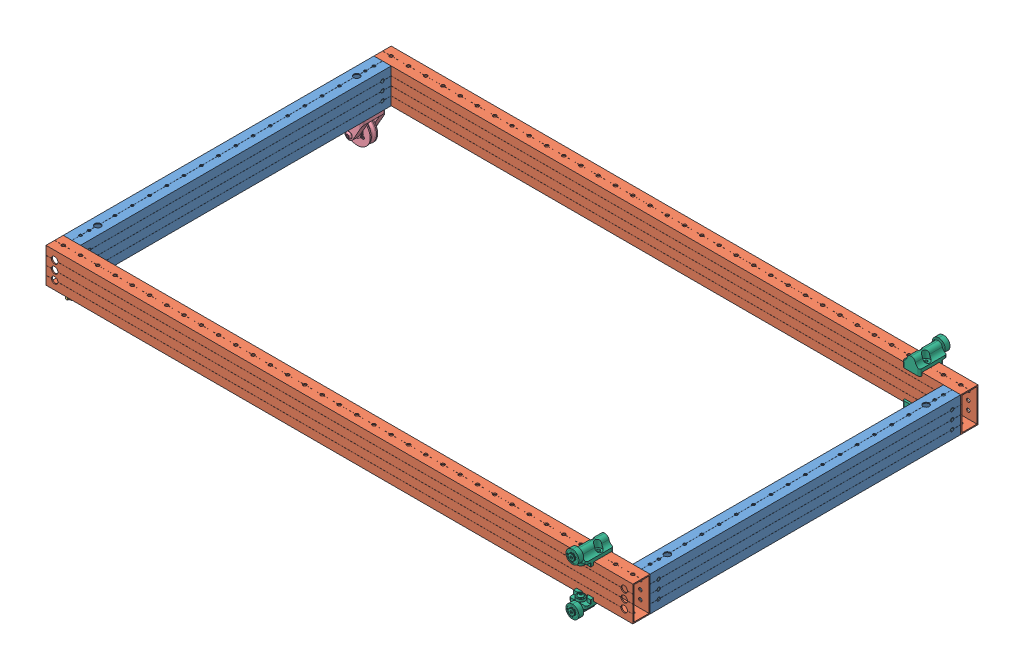
SolidWorks assembly 2 Stage, configuration Default. Lengths in mm.
Overall size (876.27 114.3 549.66).
14 component instances, 6 part files, 22 mates.
Components (placement in the parent):
- Vexpro - 1x2 18in 0.05in- 217-3425-2: Vexpro - 1x2 18in 0.05in- 217-3425 [Default] at (608.6545 998.9051 349.5436) size (25.4 50.8 457.2)
- 2 stage Vertical Versaframe-2: 2 stage Vertical Versaframe [Default] at (-254.9201 998.9051 -56.8564) x (0 0 -1) z (0 -1 0) size (25.4 863.57 50.8)
- 2 stage Vertical Versaframe-3: 2 stage Vertical Versaframe [Default] at (-254.9201 998.9051 -539.4564) x (0 0 -1) z (0 -1 0) size (25.4 863.57 50.8)
- Vexpro - 1x2 18in 0.05in- 217-3425-3: Vexpro - 1x2 18in 0.05in- 217-3425 [Default] at (-229.5201 998.9051 349.5436) size (25.4 50.8 457.2)
- String Pulley-1: String Pulley [Default] at (989.6799 998.9051 -56.8564) x (0 0 -1) z (0 1 0) size (47.02 38.1 44.45)
- MirrorString Pulley-5: MirrorString Pulley [Default] at (989.6799 998.9051 -285.4564) x (0 0 1) z (0 -1 0) size (47.02 38.1 44.45)
- Block-1: Block [Default] at (-1448.7201 998.6511 -56.8564) x (0 0 1) z (0 1 0) size (20.64 21.84 47.24)
- Block-2: Block [Default] at (-1448.7201 998.6511 -285.4564) x (0 0 -1) z (0 -1 0) size (20.64 21.84 47.24)
- Block-3: Block [Default] at (-610.5455 998.6511 -56.8564) x (0 0 1) z (0 1 0) size (20.64 21.84 47.24)
- Block-4: Block [Default] at (-610.5455 998.6511 -285.4564) x (0 0 -1) z (0 -1 0) size (20.64 21.84 47.24)
- WCP 0320-3: WCP 0320 [Default] at (-597.8201 998.9051 -577.5564) x (0 0 1) z (0 1 0) size (49.35 25.41 29.22)
- WCP 0320-4: WCP 0320 [Default] at (1700.8799 998.9051 -577.5564) x (0 0 1) z (0 -1 0) size (49.35 25.41 29.22)
- WCP 0320-5: WCP 0320 [Default] at (1700.8799 998.9051 235.2436) x (0 0 -1) z (0 1 0) size (49.35 25.41 29.22)
- WCP 0320-6: WCP 0320 [Default] at (-597.8201 998.9051 235.2436) x (0 0 -1) z (0 -1 0) size (49.35 25.41 29.22)
Mates (geometry in assembly coordinates):
- Coincident1: coincident anti-aligned: plane of Vexpro - 1x2 18in 0.05in- 217-3425-2 through (608.6545 998.9051 57.4436) normal (0 0 1); plane of 2 stage Vertical Versaframe-2 through (976.9799 1024.3051 57.4436) normal (0 0 -1)
- Coincident3: coincident aligned: plane of Vexpro - 1x2 18in 0.05in- 217-3425-2 through (595.9545 973.5051 1098.8436) normal (0 -1 0); plane of 2 stage Vertical Versaframe-2 through (976.9799 973.5051 57.4436) normal (0 -1 0)
- Coincident5: coincident anti-aligned: plane of Vexpro - 1x2 18in 0.05in- 217-3425-2 through (608.6545 998.9051 -399.7564) normal (0 0 -1); plane of 2 stage Vertical Versaframe-3 through (976.9799 1024.3051 -399.7564) normal (0 0 1)
- Coincident7: coincident aligned: plane of Vexpro - 1x2 18in 0.05in- 217-3425-2 through (595.9545 1024.3051 1098.8436) normal (0 1 0); plane of 2 stage Vertical Versaframe-3 through (976.9799 1024.3051 -425.1564) normal (0 1 0)
- Coincident8: coincident anti-aligned: plane of 2 stage Vertical Versaframe-2 through (976.9799 1024.3051 57.4436) normal (0 0 -1); plane of Vexpro - 1x2 18in 0.05in- 217-3425-3 through (-229.5201 998.9051 57.4436) normal (0 0 1)
- Coincident9: coincident aligned: plane of 2 stage Vertical Versaframe-2 through (976.9799 973.5051 57.4436) normal (0 -1 0); plane of Vexpro - 1x2 18in 0.05in- 217-3425-3 through (-242.2201 973.5051 1098.8436) normal (0 -1 0)
- Coincident10: coincident aligned: plane of 2 stage Vertical Versaframe-2 through (-242.2201 998.9051 70.1436) normal (-1 0 0); plane of Vexpro - 1x2 18in 0.05in- 217-3425-3 through (-242.2201 973.5051 1098.8436) normal (-1 0 0)
- Coincident11: coincident anti-aligned: plane of Vexpro - 1x2 18in 0.05in- 217-3425-3 through (-242.2201 973.5051 1098.8436) normal (0 -1 0); plane of String Pulley-1 through (-229.5201 973.5051 14.5811) normal (0 1 0)
- Parallel2: parallel anti-aligned: plane of Vexpro - 1x2 18in 0.05in- 217-3425-3 through (-242.2201 973.5051 1098.8436) normal (0 -1 0)
- Concentric14: concentric aligned: circle of Vexpro - 1x2 18in 0.05in- 217-3425-3; circle of Block-1
- Coincident19: coincident aligned: plane of Vexpro - 1x2 18in 0.05in- 217-3425-3 through (-229.5201 998.9051 57.4436) normal (0 0 1); plane of Block-1 through (-229.5201 998.6511 57.4436) normal (0 0 1)
- Distance1: distance = 0.254 mm anti-aligned: plane of Block-1 through (-240.4421 975.0291 38.3936) normal (0 -1 0); plane of Vexpro - 1x2 18in 0.05in- 217-3425-3 through (-229.5201 974.7751 1098.8436) normal (0 1 0)
- Concentric15: concentric anti-aligned: circle of Vexpro - 1x2 18in 0.05in- 217-3425-2; circle of Block-3
- Coincident21: coincident aligned: plane of Vexpro - 1x2 18in 0.05in- 217-3425-2 through (608.6545 998.9051 57.4436) normal (0 0 1); plane of Block-3 through (608.6545 998.6511 57.4436) normal (0 0 1)
- Distance2: distance = 0.254 mm anti-aligned: plane of Block-3 through (597.7325 975.0291 38.3936) normal (0 -1 0); plane of Vexpro - 1x2 18in 0.05in- 217-3425-2 through (608.6545 974.7751 1098.8436) normal (0 1 0)
- Coincident22: coincident aligned: plane of Vexpro - 1x2 18in 0.05in- 217-3425-2 through (621.3545 973.5051 1098.8436) normal (1 0 0); plane of 2 stage Vertical Versaframe-2 through (621.3545 998.9051 -56.8564) normal (1 0 0)
- Coincident23: coincident aligned: plane of Vexpro - 1x2 18in 0.05in- 217-3425-2 through (621.3545 973.5051 1098.8436) normal (1 0 0); plane of 2 stage Vertical Versaframe-3 through (621.3545 998.9051 -539.4564) normal (1 0 0)
- Concentric19: concentric anti-aligned: circle of Vexpro - 1x2 18in 0.05in- 217-3425-3; circle of String Pulley-1
- Parallel3: parallel aligned: plane of Vexpro - 1x2 18in 0.05in- 217-3425-3 through (-242.2201 973.5051 1098.8436) normal (-1 0 0); plane of String Pulley-1 through (-242.2201 973.5051 14.5811) normal (-1 0 0)
- Coincident24: coincident anti-aligned: plane of 2 stage Vertical Versaframe-3 through (976.9799 1024.3051 -425.1564) normal (0 1 0); plane of WCP 0320-3 through (551.5299 1024.3051 -425.2199) normal (0 -1 0)
- Concentric20: concentric anti-aligned: cylinder of WCP 0320-3 through (545.1799 1040.1801 -412.4564) axis (0 -1 0) radius 2.4892; cylinder of 2 stage Vertical Versaframe-3 through (545.1799 948.1051 -412.4564) axis (0 1 0) radius 2.4892
- Concentric21: concentric aligned: circle of 2 stage Vertical Versaframe-3; circle of WCP 0320-3
